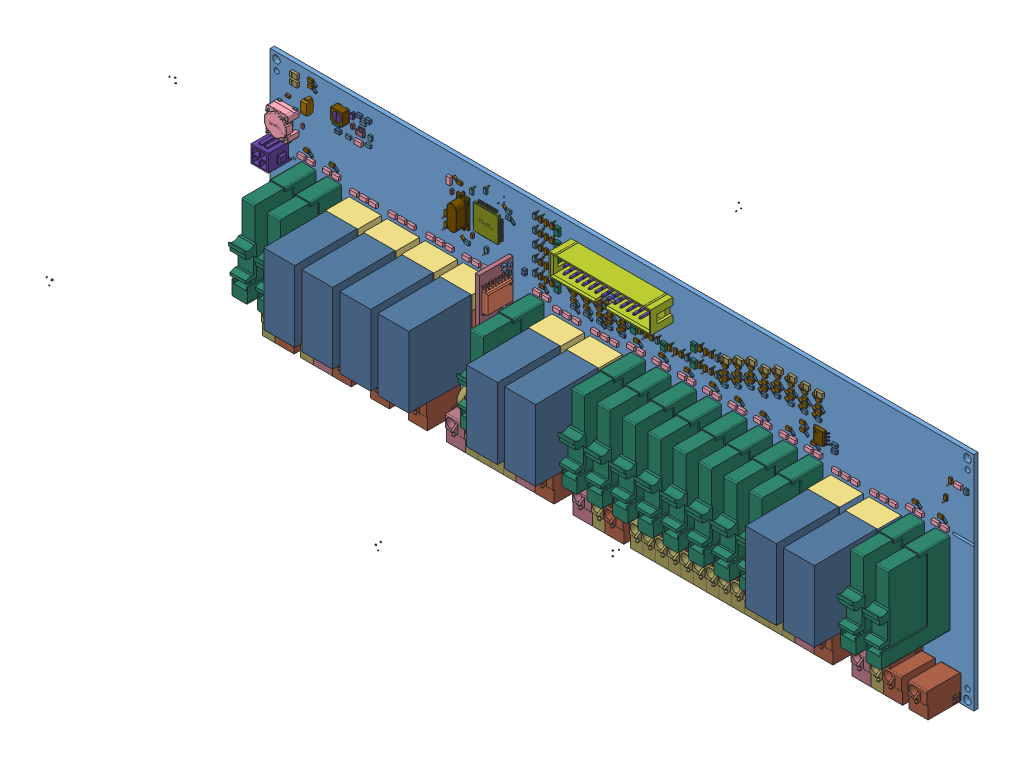
SolidWorks assembly _SC941C, configuration Default. Lengths in mm. (continued)
Components (placement in the parent): (continued)
- D33-1: D33 [Default] at origin size (1.9 2.9 0.99)
  - 1151710376-1: 1151710376 [Default] at (164.592 62.23 0) size (1.9 2.9 0.98)
    - Extruded-1: Extruded [Default] at origin size (1.9 2.9 0.98)
  - 1151710512-1: 1151710512 [Default] at (164.592 62.865 0.95) size (1.78 0.25 0.04)
    - Extruded_1-1: Extruded_1 [Default] at origin size (1.78 0.25 0.04)
- D31-1: D31 [Default] at origin size (1.9 2.9 0.99)
  - 1151710376-1: 1151710376 [Default] at (164.465 56.388 0) size (1.9 2.9 0.98)
    - Extruded-1: Extruded [Default] at origin size (1.9 2.9 0.98)
  - 1151710512-1: 1151710512 [Default] at (164.465 57.023 0.95) size (1.78 0.25 0.04)
    - Extruded_1-1: Extruded_1 [Default] at origin size (1.78 0.25 0.04)
- D29-1: D29 [Default] at origin size (1.9 2.9 0.99)
  - 1151710376-1: 1151710376 [Default] at (152.527 56.388 0) size (1.9 2.9 0.98)
    - Extruded-1: Extruded [Default] at origin size (1.9 2.9 0.98)
  - 1151710512-1: 1151710512 [Default] at (152.527 57.023 0.95) size (1.78 0.25 0.04)
    - Extruded_1-1: Extruded_1 [Default] at origin size (1.78 0.25 0.04)
- D23-1: D23 [Default] at origin size (1.9 2.9 0.99)
  - 1151710376-1: 1151710376 [Default] at (140.589 56.388 0) size (1.9 2.9 0.98)
    - Extruded-1: Extruded [Default] at origin size (1.9 2.9 0.98)
  - 1151710512-1: 1151710512 [Default] at (140.589 57.023 0.95) size (1.78 0.25 0.04)
    - Extruded_1-1: Extruded_1 [Default] at origin size (1.78 0.25 0.04)
- D22-1: D22 [Default] at origin size (2.9 1.9 0.99)
  - 905269392-1: 905269392 [Default] at (131.318 61.087 0) size (2.9 1.9 0.98)
    - Extruded_17-1: Extruded_17 [Default] at origin size (2.9 1.9 0.98)
  - 905269800-1: 905269800 [Default] at (130.683 61.087 0.95) size (0.25 1.78 0.04)
    - Extruded_18-1: Extruded_18 [Default] at origin size (0.25 1.78 0.04)
- D20-1: D20 [Default] at origin size (2.9 1.9 0.99)
  - 905269392-1: 905269392 [Default] at (136.525 61.087 0) size (2.9 1.9 0.98)
    - Extruded_17-1: Extruded_17 [Default] at origin size (2.9 1.9 0.98)
  - 905269800-1: 905269800 [Default] at (135.89 61.087 0.95) size (0.25 1.78 0.04)
    - Extruded_18-1: Extruded_18 [Default] at origin size (0.25 1.78 0.04)
- D18-1: D18 [Default] at origin size (2.9 1.9 0.99)
  - 905269392-1: 905269392 [Default] at (126.111 61.087 0) size (2.9 1.9 0.98)
    - Extruded_17-1: Extruded_17 [Default] at origin size (2.9 1.9 0.98)
  - 905269800-1: 905269800 [Default] at (126.746 61.087 0.95) size (0.25 1.78 0.04)
    - Extruded_18-1: Extruded_18 [Default] at origin size (0.25 1.78 0.04)
- D12-1: D12 [Default] at origin size (2.9 1.9 0.99)
  - 905269392-1: 905269392 [Default] at (120.904 61.087 0) size (2.9 1.9 0.98)
    - Extruded_17-1: Extruded_17 [Default] at origin size (2.9 1.9 0.98)
  - 905269800-1: 905269800 [Default] at (121.539 61.087 0.95) size (0.25 1.78 0.04)
    - Extruded_18-1: Extruded_18 [Default] at origin size (0.25 1.78 0.04)
- D10-1: D10 [Default] at origin size (1.9 2.9 0.99)
  - 1151710376-1: 1151710376 [Default] at (109.855 60.198 0) size (1.9 2.9 0.98)
    - Extruded-1: Extruded [Default] at origin size (1.9 2.9 0.98)
  - 1151710512-1: 1151710512 [Default] at (109.855 60.833 0.95) size (1.78 0.25 0.04)
    - Extruded_1-1: Extruded_1 [Default] at origin size (1.78 0.25 0.04)
- D19-1: D19 [Default] at origin size (1.9 2.9 0.99)
  - 1151710376-1: 1151710376 [Default] at (109.855 55.245 0) size (1.9 2.9 0.98)
    - Extruded-1: Extruded [Default] at origin size (1.9 2.9 0.98)
  - 1151710512-1: 1151710512 [Default] at (109.855 55.88 0.95) size (1.78 0.25 0.04)
    - Extruded_1-1: Extruded_1 [Default] at origin size (1.78 0.25 0.04)
- D16-1: D16 [Default] at origin size (1.9 2.9 0.99)
  - 1151710376-1: 1151710376 [Default] at (109.855 75.057 0) size (1.9 2.9 0.98)
    - Extruded-1: Extruded [Default] at origin size (1.9 2.9 0.98)
  - 1151710512-1: 1151710512 [Default] at (109.855 75.692 0.95) size (1.78 0.25 0.04)
    - Extruded_1-1: Extruded_1 [Default] at origin size (1.78 0.25 0.04)
- D13-1: D13 [Default] at origin size (1.9 2.9 0.99)
  - 1151710376-1: 1151710376 [Default] at (109.855 65.151 0) size (1.9 2.9 0.98)
    - Extruded-1: Extruded [Default] at origin size (1.9 2.9 0.98)
  - 1151710512-1: 1151710512 [Default] at (109.855 65.786 0.95) size (1.78 0.25 0.04)
    - Extruded_1-1: Extruded_1 [Default] at origin size (1.78 0.25 0.04)
- D11-1: D11 [Default] at origin size (1.9 2.9 0.99)
  - 1151710376-1: 1151710376 [Default] at (109.855 70.104 0) size (1.9 2.9 0.98)
    - Extruded-1: Extruded [Default] at origin size (1.9 2.9 0.98)
  - 1151710512-1: 1151710512 [Default] at (109.855 70.739 0.95) size (1.78 0.25 0.04)
    - Extruded_1-1: Extruded_1 [Default] at origin size (1.78 0.25 0.04)
- D32-1: D32 [Default] at origin size (104.77 29.62 23.48)
  - SW3dPS-transistor_SOT233_4-1: SW3dPS-transistor_SOT233_4 [Default] at (101.3713 26.7469 -21.9) x (-1 0 0) z (0 1 0) size (2.9 1.1 1.6)
  - SW3dPS-transistor_SOT233_5-1: SW3dPS-transistor_SOT233_5 [Default] at (0.1014 0.0267 -0.0219) x (-1 0 0) z (0 1 0) size (2.18 2.18 2.18)
  - SW3dPS-transistor_SOT233_6-1: SW3dPS-transistor_SOT233_6 [Default] at (0.0001 0 0) x (-1 0 0) z (0 1 0) size (2.18 2.18 2.18)
  - SW3dPS-transistor_SOT233_7-1: SW3dPS-transistor_SOT233_7 [Default] x (-1 0 0) z (0 1 0) size (2.18 2.18 2.18)
- D30-1: D30 [Default] at origin size (94.62 29.62 23.48)
  - SW3dPS-transistor_SOT233_4-1: SW3dPS-transistor_SOT233_4 [Default] at (91.2113 26.7469 -21.9) x (-1 0 0) z (0 1 0) size (2.9 1.1 1.6)
  - SW3dPS-transistor_SOT233_5-1: SW3dPS-transistor_SOT233_5 [Default] at (0.0912 0.0267 -0.0219) x (-1 0 0) z (0 1 0) size (2.18 2.18 2.18)
  - SW3dPS-transistor_SOT233_6-1: SW3dPS-transistor_SOT233_6 [Default] at (0.0001 0 0) x (-1 0 0) z (0 1 0) size (2.18 2.18 2.18)
  - SW3dPS-transistor_SOT233_7-1: SW3dPS-transistor_SOT233_7 [Default] x (-1 0 0) z (0 1 0) size (2.18 2.18 2.18)
- D48-1: D48 [Default] at origin size (2.9 1.9 0.99)
  - 905269392-1: 905269392 [Default] at (193.294 68.707 0) size (2.9 1.9 0.98)
    - Extruded_17-1: Extruded_17 [Default] at origin size (2.9 1.9 0.98)
  - 905269800-1: 905269800 [Default] at (192.659 68.707 0.95) size (0.25 1.78 0.04)
    - Extruded_18-1: Extruded_18 [Default] at origin size (0.25 1.78 0.04)
- D46-1: D46 [Default] at origin size (2.9 1.9 0.99)
  - 905269392-1: 905269392 [Default] at (198.501 70.993 0) size (2.9 1.9 0.98)
    - Extruded_17-1: Extruded_17 [Default] at origin size (2.9 1.9 0.98)
  - 905269800-1: 905269800 [Default] at (197.866 70.993 0.95) size (0.25 1.78 0.04)
    - Extruded_18-1: Extruded_18 [Default] at origin size (0.25 1.78 0.04)
- D44-1: D44 [Default] at origin size (171.7 27.55 23.48)
  - SW3dPS-transistor_SOT233_4-1: SW3dPS-transistor_SOT233_4 [Default] at (168.3638 24.6832 -21.9) x (-1 0 0) z (0 1 0) size (2.9 1.1 1.6)
  - SW3dPS-transistor_SOT233_5-1: SW3dPS-transistor_SOT233_5 [Default] at (0.1684 0.0247 -0.0219) x (-1 0 0) z (0 1 0) size (2.18 2.18 2.18)
  - SW3dPS-transistor_SOT233_6-1: SW3dPS-transistor_SOT233_6 [Default] at (0.0002 0 0) x (-1 0 0) z (0 1 0) size (2.18 2.18 2.18)
  - SW3dPS-transistor_SOT233_7-1: SW3dPS-transistor_SOT233_7 [Default] x (-1 0 0) z (0 1 0) size (2.18 2.18 2.18)
- D42-1: D42 [Default] at origin size (156.47 27.55 23.48)
  - SW3dPS-transistor_SOT233_4-1: SW3dPS-transistor_SOT233_4 [Default] at (153.1238 24.6832 -21.9) x (-1 0 0) z (0 1 0) size (2.9 1.1 1.6)
  - SW3dPS-transistor_SOT233_5-1: SW3dPS-transistor_SOT233_5 [Default] at (0.1531 0.0247 -0.0219) x (-1 0 0) z (0 1 0) size (2.18 2.18 2.18)
  - SW3dPS-transistor_SOT233_6-1: SW3dPS-transistor_SOT233_6 [Default] at (0.0002 0 0) x (-1 0 0) z (0 1 0) size (2.18 2.18 2.18)
  - SW3dPS-transistor_SOT233_7-1: SW3dPS-transistor_SOT233_7 [Default] x (-1 0 0) z (0 1 0) size (2.18 2.18 2.18)
- D26-1: D26 [Default] at origin size (60.05 27.6 23.48)
  - SW3dPS-transistor_SOT233_4-1: SW3dPS-transistor_SOT233_4 [Default] at (56.6038 24.7282 -21.9) x (-1 0 0) z (0 1 0) size (2.9 1.1 1.6)
  - SW3dPS-transistor_SOT233_5-1: SW3dPS-transistor_SOT233_5 [Default] at (0.0566 0.0247 -0.0219) x (-1 0 0) z (0 1 0) size (2.18 2.18 2.18)
  - SW3dPS-transistor_SOT233_6-1: SW3dPS-transistor_SOT233_6 [Default] at (0.0001 0 0) x (-1 0 0) z (0 1 0) size (2.18 2.18 2.18)
  - SW3dPS-transistor_SOT233_7-1: SW3dPS-transistor_SOT233_7 [Default] x (-1 0 0) z (0 1 0) size (2.18 2.18 2.18)
- D25-1: D25 [Default] at origin size (44.82 27.6 23.48)
  - SW3dPS-transistor_SOT233_4-1: SW3dPS-transistor_SOT233_4 [Default] at (41.3638 24.7282 -21.9) x (-1 0 0) z (0 1 0) size (2.9 1.1 1.6)
  - SW3dPS-transistor_SOT233_5-1: SW3dPS-transistor_SOT233_5 [Default] at (0.0414 0.0247 -0.0219) x (-1 0 0) z (0 1 0) size (2.18 2.18 2.18)
  - SW3dPS-transistor_SOT233_6-1: SW3dPS-transistor_SOT233_6 [Default] at (0 0 0) x (-1 0 0) z (0 1 0) size (2.18 2.18 2.18)
  - SW3dPS-transistor_SOT233_7-1: SW3dPS-transistor_SOT233_7 [Default] x (-1 0 0) z (0 1 0) size (2.18 2.18 2.18)
- D21-1: D21 [Default] at origin size (8.51 27.6 23.48)
  - SW3dPS-transistor_SOT233_4-1: SW3dPS-transistor_SOT233_4 [Default] at (5.0101 24.7282 -21.9) x (-1 0 0) z (0 1 0) size (2.9 1.1 1.6)
  - SW3dPS-transistor_SOT233_5-1: SW3dPS-transistor_SOT233_5 [Default] at (0.005 0.0247 -0.0219) x (-1 0 0) z (0 1 0) size (2.18 2.18 2.18)
  - SW3dPS-transistor_SOT233_6-1: SW3dPS-transistor_SOT233_6 [Default] at (0 0 0) x (-1 0 0) z (0 1 0) size (2.18 2.18 2.18)
  - SW3dPS-transistor_SOT233_7-1: SW3dPS-transistor_SOT233_7 [Default] x (-1 0 0) z (0 1 0) size (2.18 2.18 2.18)
- D17-1: D17 [Default] at origin size (12.91 27.55 23.48)
  - SW3dPS-transistor_SOT233_4-1: SW3dPS-transistor_SOT233_4 [Default] at (-9.4362 24.6832 -21.9) x (-1 0 0) z (0 1 0) size (2.9 1.1 1.6)
  - SW3dPS-transistor_SOT233_5-1: SW3dPS-transistor_SOT233_5 [Default] at (-0.0094 0.0247 -0.0219) x (-1 0 0) z (0 1 0) size (2.18 2.18 2.18)
  - SW3dPS-transistor_SOT233_6-1: SW3dPS-transistor_SOT233_6 [Default] at (0 0 0) x (-1 0 0) z (0 1 0) size (2.18 2.18 2.18)
  - SW3dPS-transistor_SOT233_7-1: SW3dPS-transistor_SOT233_7 [Default] x (-1 0 0) z (0 1 0) size (2.18 2.18 2.18)
- D14-1: D14 [Default] at origin size (28.15 27.55 23.48)
  - SW3dPS-transistor_SOT233_4-1: SW3dPS-transistor_SOT233_4 [Default] at (-24.6762 24.6832 -21.9) x (-1 0 0) z (0 1 0) size (2.9 1.1 1.6)
  - SW3dPS-transistor_SOT233_5-1: SW3dPS-transistor_SOT233_5 [Default] at (-0.0247 0.0247 -0.0219) x (-1 0 0) z (0 1 0) size (2.18 2.18 2.18)
  - SW3dPS-transistor_SOT233_6-1: SW3dPS-transistor_SOT233_6 [Default] at (0 0 0) x (-1 0 0) z (0 1 0) size (2.18 2.18 2.18)
  - SW3dPS-transistor_SOT233_7-1: SW3dPS-transistor_SOT233_7 [Default] x (-1 0 0) z (0 1 0) size (2.18 2.18 2.18)
- D9-1: D9 [Default] at origin size (43.39 27.55 23.48)
  - SW3dPS-transistor_SOT233_4-1: SW3dPS-transistor_SOT233_4 [Default] at (-39.9162 24.6832 -21.9) x (-1 0 0) z (0 1 0) size (2.9 1.1 1.6)
  - SW3dPS-transistor_SOT233_5-1: SW3dPS-transistor_SOT233_5 [Default] at (-0.0399 0.0247 -0.0219) x (-1 0 0) z (0 1 0) size (2.18 2.18 2.18)
  - SW3dPS-transistor_SOT233_6-1: SW3dPS-transistor_SOT233_6 [Default] at (0 0 0) x (-1 0 0) z (0 1 0) size (2.18 2.18 2.18)
  - SW3dPS-transistor_SOT233_7-1: SW3dPS-transistor_SOT233_7 [Default] x (-1 0 0) z (0 1 0) size (2.18 2.18 2.18)
- C26-1: C26 [Default] at origin size (1.97 3.3 0.78)
  - SW3dPS-0805_SMD_Capacitor-1: SW3dPS-0805_SMD_Capacitor [Default] at (67.437 58.9279 0) x (0 -1 0) z (-1 0 0) size (2 0.78 1.25)
  - 905260688-1: 905260688 [Default] at (68.072 60.5949 0) size (1.43 1.11 0.76)
    - Extruded_13-1: Extruded_13 [Default] at origin size (1.43 1.11 0.76)
  - 905261368-1: 905261368 [Default] at (68.0323 60.4758 0) size (1.51 1.51 0.76)
    - Extruded_12-1: Extruded_12 [Default] at origin size (1.51 1.51 0.76)
  - 905262864-1: 905262864 [Default] at (68.1117 60.7139 0) size (1.35 1.03 0.76)
    - Extruded_11-1: Extruded_11 [Default] at origin size (1.35 1.03 0.76)
- C24-1: C24 [Default] at origin size (1.97 3.3 0.78)
  - SW3dPS-0805_SMD_Capacitor-1: SW3dPS-0805_SMD_Capacitor [Default] at (67.437 54.8639 0) x (0 -1 0) z (-1 0 0) size (2 0.78 1.25)
  - 905260688-1: 905260688 [Default] at (68.072 56.5309 0) size (1.43 1.11 0.76)
    - Extruded_13-1: Extruded_13 [Default] at origin size (1.43 1.11 0.76)
  - 905261368-1: 905261368 [Default] at (68.0323 56.4118 0) size (1.51 1.51 0.76)
    - Extruded_12-1: Extruded_12 [Default] at origin size (1.51 1.51 0.76)
  - 905262864-1: 905262864 [Default] at (68.1117 56.6499 0) size (1.35 1.03 0.76)
    - Extruded_11-1: Extruded_11 [Default] at origin size (1.35 1.03 0.76)
- C17-1: C17 [Default] at origin size (3.3 1.97 0.78)
  - SW3dPS-0805_SMD_Capacitor-1: SW3dPS-0805_SMD_Capacitor [Default] at (90.2971 72.009 0) x (1 0 0) z (0 -1 0) size (2 0.78 1.25)
  - 905266536-1: 905266536 [Default] at (88.6301 72.644 0) size (1.11 1.43 0.76)
    - Extruded_16-1: Extruded_16 [Default] at origin size (1.11 1.43 0.76)
  - 905263816-1: 905263816 [Default] at (88.7492 72.6043 0) size (1.51 1.51 0.76)
    - Extruded_15-1: Extruded_15 [Default] at origin size (1.51 1.51 0.76)
  - 905266264-1: 905266264 [Default] at (88.5111 72.6837 0) size (1.03 1.35 0.76)
    - Extruded_14-1: Extruded_14 [Default] at origin size (1.03 1.35 0.76)
- C19-1: C19 [Default] at origin size (1.97 3.3 0.78)
  - SW3dPS-0805_SMD_Capacitor-1: SW3dPS-0805_SMD_Capacitor [Default] at (81.0298 74.5344 0) x (0 -1 0) z (-1 0 0) size (2 0.78 1.25)
  - 905260688-1: 905260688 [Default] at (81.6648 76.2014 0) size (1.43 1.11 0.76)
    - Extruded_13-1: Extruded_13 [Default] at origin size (1.43 1.11 0.76)
  - 905261368-1: 905261368 [Default] at (81.6251 76.0823 0) size (1.51 1.51 0.76)
    - Extruded_12-1: Extruded_12 [Default] at origin size (1.51 1.51 0.76)
  - 905262864-1: 905262864 [Default] at (81.7045 76.3204 0) size (1.35 1.03 0.76)
    - Extruded_11-1: Extruded_11 [Default] at origin size (1.35 1.03 0.76)
- C25-1: C25 [Default] at origin size (3.3 1.97 0.78)
  - SW3dPS-0805_SMD_Capacitor-1: SW3dPS-0805_SMD_Capacitor [Default] at (90.2969 69.723 0) x (-1 0 0) z (0 1 0) size (2 0.78 1.25)
  - 905265720-1: 905265720 [Default] at (91.9639 69.088 0) size (1.11 1.43 0.76)
    - Extruded_4-1: Extruded_4 [Default] at origin size (1.11 1.43 0.76)
  - 905275240-1: 905275240 [Default] at (91.8448 69.1277 0) size (1.51 1.51 0.76)
    - Extruded_3-1: Extruded_3 [Default] at origin size (1.51 1.51 0.76)
  - 905261096-1: 905261096 [Default] at (92.0829 69.0483 0) size (1.03 1.35 0.76)
    - Extruded_2-1: Extruded_2 [Default] at origin size (1.03 1.35 0.76)
- C21-1: C21 [Default] at origin size (3.3 1.97 0.78)
  - SW3dPS-0805_SMD_Capacitor-1: SW3dPS-0805_SMD_Capacitor [Default] at (73.6601 52.832 0) x (1 0 0) z (0 -1 0) size (2 0.78 1.25)
  - 905266536-1: 905266536 [Default] at (71.9931 53.467 0) size (1.11 1.43 0.76)
    - Extruded_16-1: Extruded_16 [Default] at origin size (1.11 1.43 0.76)
  - 905263816-1: 905263816 [Default] at (72.1122 53.4273 0) size (1.51 1.51 0.76)
    - Extruded_15-1: Extruded_15 [Default] at origin size (1.51 1.51 0.76)
  - 905266264-1: 905266264 [Default] at (71.8741 53.5067 0) size (1.03 1.35 0.76)
    - Extruded_14-1: Extruded_14 [Default] at origin size (1.03 1.35 0.76)
- C18-1: C18 [Default] at origin size (1.97 3.3 0.78)
  - SW3dPS-0805_SMD_Capacitor-1: SW3dPS-0805_SMD_Capacitor [Default] at (75.4736 71.5181 0) x (0 -1 0) z (-1 0 0) size (2 0.78 1.25)
  - 905260688-1: 905260688 [Default] at (76.1086 73.1851 0) size (1.43 1.11 0.76)
    - Extruded_13-1: Extruded_13 [Default] at origin size (1.43 1.11 0.76)
  - 905261368-1: 905261368 [Default] at (76.0689 73.066 0) size (1.51 1.51 0.76)
    - Extruded_12-1: Extruded_12 [Default] at origin size (1.51 1.51 0.76)
  - 905262864-1: 905262864 [Default] at (76.1483 73.3041 0) size (1.35 1.03 0.76)
    - Extruded_11-1: Extruded_11 [Default] at origin size (1.35 1.03 0.76)
- C20-1: C20 [Default] at origin size (1.97 3.3 0.78)
  - SW3dPS-0805_SMD_Capacitor-1: SW3dPS-0805_SMD_Capacitor [Default] at (81.3473 54.1828 0) x (0 1 0) z (1 0 0) size (2 0.78 1.25)
  - 905266128-1: 905266128 [Default] at (80.7123 52.5158 0) size (1.43 1.11 0.76)
    - Extruded_10-1: Extruded_10 [Default] at origin size (1.43 1.11 0.76)
  - 905260416-1: 905260416 [Default] at (80.752 52.6349 0) size (1.51 1.51 0.76)
    - Extruded_9-1: Extruded_9 [Default] at origin size (1.51 1.51 0.76)
  - 905261640-1: 905261640 [Default] at (80.6726 52.3968 0) size (1.35 1.03 0.76)
    - Extruded_8-1: Extruded_8 [Default] at origin size (1.35 1.03 0.76)
- C37-1: C37 [Default] at origin size (3.3 1.97 0.78)
  - SW3dPS-0805_SMD_Capacitor-1: SW3dPS-0805_SMD_Capacitor [Default] at (192.7861 59.563 0) x (1 0 0) z (0 -1 0) size (2 0.78 1.25)
  - 905266536-1: 905266536 [Default] at (191.1191 60.198 0) size (1.11 1.43 0.76)
    - Extruded_16-1: Extruded_16 [Default] at origin size (1.11 1.43 0.76)
  - 905263816-1: 905263816 [Default] at (191.2382 60.1583 0) size (1.51 1.51 0.76)
    - Extruded_15-1: Extruded_15 [Default] at origin size (1.51 1.51 0.76)
  - 905266264-1: 905266264 [Default] at (191.0001 60.2377 0) size (1.03 1.35 0.76)
    - Extruded_14-1: Extruded_14 [Default] at origin size (1.03 1.35 0.76)
- C36-1: C36 [Default] at origin size (3.3 1.97 0.78)
  - SW3dPS-0805_SMD_Capacitor-1: SW3dPS-0805_SMD_Capacitor [Default] at (197.9931 61.849 0) x (1 0 0) z (0 -1 0) size (2 0.78 1.25)
  - 905266536-1: 905266536 [Default] at (196.3261 62.484 0) size (1.11 1.43 0.76)
    - Extruded_16-1: Extruded_16 [Default] at origin size (1.11 1.43 0.76)
  - 905263816-1: 905263816 [Default] at (196.4452 62.4443 0) size (1.51 1.51 0.76)
    - Extruded_15-1: Extruded_15 [Default] at origin size (1.51 1.51 0.76)
  - 905266264-1: 905266264 [Default] at (196.2071 62.5237 0) size (1.03 1.35 0.76)
    - Extruded_14-1: Extruded_14 [Default] at origin size (1.03 1.35 0.76)
- C35-1: C35 [Default] at origin size (3.3 1.97 0.78)
  - SW3dPS-0805_SMD_Capacitor-1: SW3dPS-0805_SMD_Capacitor [Default] at (187.3251 59.563 0) x (1 0 0) z (0 -1 0) size (2 0.78 1.25)
  - 905266536-1: 905266536 [Default] at (185.6581 60.198 0) size (1.11 1.43 0.76)
    - Extruded_16-1: Extruded_16 [Default] at origin size (1.11 1.43 0.76)
  - 905263816-1: 905263816 [Default] at (185.7772 60.1583 0) size (1.51 1.51 0.76)
    - Extruded_15-1: Extruded_15 [Default] at origin size (1.51 1.51 0.76)
  - 905266264-1: 905266264 [Default] at (185.5391 60.2377 0) size (1.03 1.35 0.76)
    - Extruded_14-1: Extruded_14 [Default] at origin size (1.03 1.35 0.76)
- C34-1: C34 [Default] at origin size (3.3 1.97 0.78)
  - SW3dPS-0805_SMD_Capacitor-1: SW3dPS-0805_SMD_Capacitor [Default] at (203.4541 61.849 0) x (1 0 0) z (0 -1 0) size (2 0.78 1.25)
  - 905266536-1: 905266536 [Default] at (201.7871 62.484 0) size (1.11 1.43 0.76)
    - Extruded_16-1: Extruded_16 [Default] at origin size (1.11 1.43 0.76)
  - 905263816-1: 905263816 [Default] at (201.9062 62.4443 0) size (1.51 1.51 0.76)
    - Extruded_15-1: Extruded_15 [Default] at origin size (1.51 1.51 0.76)
  - 905266264-1: 905266264 [Default] at (201.6681 62.5237 0) size (1.03 1.35 0.76)
    - Extruded_14-1: Extruded_14 [Default] at origin size (1.03 1.35 0.76)
- C33-1: C33 [Default] at origin size (3.3 1.97 0.78)
  - SW3dPS-0805_SMD_Capacitor-1: SW3dPS-0805_SMD_Capacitor [Default] at (182.1181 57.277 0) x (1 0 0) z (0 -1 0) size (2 0.78 1.25)
  - 905266536-1: 905266536 [Default] at (180.4511 57.912 0) size (1.11 1.43 0.76)
    - Extruded_16-1: Extruded_16 [Default] at origin size (1.11 1.43 0.76)
  - 905263816-1: 905263816 [Default] at (180.5702 57.8723 0) size (1.51 1.51 0.76)
    - Extruded_15-1: Extruded_15 [Default] at origin size (1.51 1.51 0.76)
  - 905266264-1: 905266264 [Default] at (180.3321 57.9517 0) size (1.03 1.35 0.76)
    - Extruded_14-1: Extruded_14 [Default] at origin size (1.03 1.35 0.76)
- C32-1: C32 [Default] at origin size (3.3 1.97 0.78)
  - SW3dPS-0805_SMD_Capacitor-1: SW3dPS-0805_SMD_Capacitor [Default] at (208.9151 61.849 0) x (1 0 0) z (0 -1 0) size (2 0.78 1.25)
  - 905266536-1: 905266536 [Default] at (207.2481 62.484 0) size (1.11 1.43 0.76)
    - Extruded_16-1: Extruded_16 [Default] at origin size (1.11 1.43 0.76)
  - 905263816-1: 905263816 [Default] at (207.3672 62.4443 0) size (1.51 1.51 0.76)
    - Extruded_15-1: Extruded_15 [Default] at origin size (1.51 1.51 0.76)
  - 905266264-1: 905266264 [Default] at (207.1291 62.5237 0) size (1.03 1.35 0.76)
    - Extruded_14-1: Extruded_14 [Default] at origin size (1.03 1.35 0.76)
- C31-1: C31 [Default] at origin size (3.3 1.97 0.78)
  - SW3dPS-0805_SMD_Capacitor-1: SW3dPS-0805_SMD_Capacitor [Default] at (176.9111 54.991 0) x (1 0 0) z (0 -1 0) size (2 0.78 1.25)
  - 905266536-1: 905266536 [Default] at (175.2441 55.626 0) size (1.11 1.43 0.76)
    - Extruded_16-1: Extruded_16 [Default] at origin size (1.11 1.43 0.76)
  - 905263816-1: 905263816 [Default] at (175.3632 55.5863 0) size (1.51 1.51 0.76)
    - Extruded_15-1: Extruded_15 [Default] at origin size (1.51 1.51 0.76)
  - 905266264-1: 905266264 [Default] at (175.1251 55.6657 0) size (1.03 1.35 0.76)
    - Extruded_14-1: Extruded_14 [Default] at origin size (1.03 1.35 0.76)
- C30-1: C30 [Default] at origin size (3.3 1.97 0.78)
  - SW3dPS-0805_SMD_Capacitor-1: SW3dPS-0805_SMD_Capacitor [Default] at (214.3761 61.849 0) x (1 0 0) z (0 -1 0) size (2 0.78 1.25)
  - 905266536-1: 905266536 [Default] at (212.7091 62.484 0) size (1.11 1.43 0.76)
    - Extruded_16-1: Extruded_16 [Default] at origin size (1.11 1.43 0.76)
  - 905263816-1: 905263816 [Default] at (212.8282 62.4443 0) size (1.51 1.51 0.76)
    - Extruded_15-1: Extruded_15 [Default] at origin size (1.51 1.51 0.76)
  - 905266264-1: 905266264 [Default] at (212.5901 62.5237 0) size (1.03 1.35 0.76)
    - Extruded_14-1: Extruded_14 [Default] at origin size (1.03 1.35 0.76)
- C29-1: C29 [Default] at origin size (1.97 3.3 0.78)
  - SW3dPS-0805_SMD_Capacitor-1: SW3dPS-0805_SMD_Capacitor [Default] at (173.736 62.7379 0) x (0 -1 0) z (-1 0 0) size (2 0.78 1.25)
  - 905260688-1: 905260688 [Default] at (174.371 64.4049 0) size (1.43 1.11 0.76)
    - Extruded_13-1: Extruded_13 [Default] at origin size (1.43 1.11 0.76)
  - 905261368-1: 905261368 [Default] at (174.3313 64.2858 0) size (1.51 1.51 0.76)
    - Extruded_12-1: Extruded_12 [Default] at origin size (1.51 1.51 0.76)
  - 905262864-1: 905262864 [Default] at (174.4107 64.5239 0) size (1.35 1.03 0.76)
    - Extruded_11-1: Extruded_11 [Default] at origin size (1.35 1.03 0.76)
- C28-1: C28 [Default] at origin size (1.97 3.3 0.78)
  - SW3dPS-0805_SMD_Capacitor-1: SW3dPS-0805_SMD_Capacitor [Default] at (173.609 56.8959 0) x (0 -1 0) z (-1 0 0) size (2 0.78 1.25)
  - 905260688-1: 905260688 [Default] at (174.244 58.5629 0) size (1.43 1.11 0.76)
    - Extruded_13-1: Extruded_13 [Default] at origin size (1.43 1.11 0.76)
  - 905261368-1: 905261368 [Default] at (174.2043 58.4438 0) size (1.51 1.51 0.76)
    - Extruded_12-1: Extruded_12 [Default] at origin size (1.51 1.51 0.76)
  - 905262864-1: 905262864 [Default] at (174.2837 58.6819 0) size (1.35 1.03 0.76)
    - Extruded_11-1: Extruded_11 [Default] at origin size (1.35 1.03 0.76)
- C16-1: C16 [Default] at origin size (1.97 3.3 0.78)
  - SW3dPS-0805_SMD_Capacitor-1: SW3dPS-0805_SMD_Capacitor [Default] at (149.733 56.8959 0) x (0 -1 0) z (-1 0 0) size (2 0.78 1.25)
  - 905260688-1: 905260688 [Default] at (150.368 58.5629 0) size (1.43 1.11 0.76)
    - Extruded_13-1: Extruded_13 [Default] at origin size (1.43 1.11 0.76)
  - 905261368-1: 905261368 [Default] at (150.3283 58.4438 0) size (1.51 1.51 0.76)
    - Extruded_12-1: Extruded_12 [Default] at origin size (1.51 1.51 0.76)
  - 905262864-1: 905262864 [Default] at (150.4077 58.6819 0) size (1.35 1.03 0.76)
    - Extruded_11-1: Extruded_11 [Default] at origin size (1.35 1.03 0.76)
- C14-1: C14 [Default] at origin size (3.3 1.97 0.78)
  - SW3dPS-0805_SMD_Capacitor-1: SW3dPS-0805_SMD_Capacitor [Default] at (130.8101 51.9431 0) x (1 0 0) z (0 -1 0) size (2 0.78 1.25)
  - 905266536-1: 905266536 [Default] at (129.1431 52.578 0) size (1.11 1.43 0.76)
    - Extruded_16-1: Extruded_16 [Default] at origin size (1.11 1.43 0.76)
  - 905263816-1: 905263816 [Default] at (129.2622 52.5383 0) size (1.51 1.51 0.76)
    - Extruded_15-1: Extruded_15 [Default] at origin size (1.51 1.51 0.76)
  - 905266264-1: 905266264 [Default] at (129.0241 52.6177 0) size (1.03 1.35 0.76)
    - Extruded_14-1: Extruded_14 [Default] at origin size (1.03 1.35 0.76)
- C13-1: C13 [Default] at origin size (3.3 1.97 0.78)
  - SW3dPS-0805_SMD_Capacitor-1: SW3dPS-0805_SMD_Capacitor [Default] at (136.0171 51.9431 0) x (1 0 0) z (0 -1 0) size (2 0.78 1.25)
  - 905266536-1: 905266536 [Default] at (134.3501 52.578 0) size (1.11 1.43 0.76)
    - Extruded_16-1: Extruded_16 [Default] at origin size (1.11 1.43 0.76)
  - 905263816-1: 905263816 [Default] at (134.4692 52.5383 0) size (1.51 1.51 0.76)
    - Extruded_15-1: Extruded_15 [Default] at origin size (1.51 1.51 0.76)
  - 905266264-1: 905266264 [Default] at (134.2311 52.6177 0) size (1.03 1.35 0.76)
    - Extruded_14-1: Extruded_14 [Default] at origin size (1.03 1.35 0.76)
- C7_1-1: C7_1 [Default] at origin size (3.3 1.97 0.78)
  - SW3dPS-0805_SMD_Capacitor-1: SW3dPS-0805_SMD_Capacitor [Default] at (121.4119 51.943 0) x (-1 0 0) z (0 1 0) size (2 0.78 1.25)
  - 905265720-1: 905265720 [Default] at (123.0789 51.308 0) size (1.11 1.43 0.76)
    - Extruded_4-1: Extruded_4 [Default] at origin size (1.11 1.43 0.76)
  - 905275240-1: 905275240 [Default] at (122.9598 51.3477 0) size (1.51 1.51 0.76)
    - Extruded_3-1: Extruded_3 [Default] at origin size (1.51 1.51 0.76)
  - 905261096-1: 905261096 [Default] at (123.1979 51.2683 0) size (1.03 1.35 0.76)
    - Extruded_2-1: Extruded_2 [Default] at origin size (1.03 1.35 0.76)
- C5_1-1: C5_1 [Default] at origin size (1.97 3.3 0.78)
  - SW3dPS-0805_SMD_Capacitor-1: SW3dPS-0805_SMD_Capacitor [Default] at (100.711 60.7059 0) x (0 -1 0) z (-1 0 0) size (2 0.78 1.25)
  - 905260688-1: 905260688 [Default] at (101.346 62.3729 0) size (1.43 1.11 0.76)
    - Extruded_13-1: Extruded_13 [Default] at origin size (1.43 1.11 0.76)
  - 905261368-1: 905261368 [Default] at (101.3063 62.2538 0) size (1.51 1.51 0.76)
    - Extruded_12-1: Extruded_12 [Default] at origin size (1.51 1.51 0.76)
  - 905262864-1: 905262864 [Default] at (101.3857 62.4919 0) size (1.35 1.03 0.76)
    - Extruded_11-1: Extruded_11 [Default] at origin size (1.35 1.03 0.76)
- C27-1: C27 [Default] at origin size (1.97 3.3 0.78)
  - SW3dPS-0805_SMD_Capacitor-1: SW3dPS-0805_SMD_Capacitor [Default] at (161.671 56.8959 0) x (0 -1 0) z (-1 0 0) size (2 0.78 1.25)
  - 905260688-1: 905260688 [Default] at (162.306 58.5629 0) size (1.43 1.11 0.76)
    - Extruded_13-1: Extruded_13 [Default] at origin size (1.43 1.11 0.76)
  - 905261368-1: 905261368 [Default] at (162.2663 58.4438 0) size (1.51 1.51 0.76)
    - Extruded_12-1: Extruded_12 [Default] at origin size (1.51 1.51 0.76)
  - 905262864-1: 905262864 [Default] at (162.3457 58.6819 0) size (1.35 1.03 0.76)
    - Extruded_11-1: Extruded_11 [Default] at origin size (1.35 1.03 0.76)
- C11-1: C11 [Default] at origin size (3.3 1.97 0.78)
  - SW3dPS-0805_SMD_Capacitor-1: SW3dPS-0805_SMD_Capacitor [Default] at (126.6189 51.943 0) x (-1 0 0) z (0 1 0) size (2 0.78 1.25)
  - 905265720-1: 905265720 [Default] at (128.2859 51.308 0) size (1.11 1.43 0.76)
    - Extruded_4-1: Extruded_4 [Default] at origin size (1.11 1.43 0.76)
  - 905275240-1: 905275240 [Default] at (128.1668 51.3477 0) size (1.51 1.51 0.76)
    - Extruded_3-1: Extruded_3 [Default] at origin size (1.51 1.51 0.76)
  - 905261096-1: 905261096 [Default] at (128.4049 51.2683 0) size (1.03 1.35 0.76)
    - Extruded_2-1: Extruded_2 [Default] at origin size (1.03 1.35 0.76)
- C12-1: C12 [Default] at origin size (1.97 3.3 0.78)
  - SW3dPS-0805_SMD_Capacitor-1: SW3dPS-0805_SMD_Capacitor [Default] at (100.711 55.7529 0) x (0 -1 0) z (-1 0 0) size (2 0.78 1.25)
  - 905260688-1: 905260688 [Default] at (101.346 57.4199 0) size (1.43 1.11 0.76)
    - Extruded_13-1: Extruded_13 [Default] at origin size (1.43 1.11 0.76)
  - 905261368-1: 905261368 [Default] at (101.3063 57.3008 0) size (1.51 1.51 0.76)
    - Extruded_12-1: Extruded_12 [Default] at origin size (1.51 1.51 0.76)
  - 905262864-1: 905262864 [Default] at (101.3857 57.5389 0) size (1.35 1.03 0.76)
    - Extruded_11-1: Extruded_11 [Default] at origin size (1.35 1.03 0.76)
- C10-1: C10 [Default] at origin size (1.97 3.3 0.78)
  - SW3dPS-0805_SMD_Capacitor-1: SW3dPS-0805_SMD_Capacitor [Default] at (100.711 75.5649 0) x (0 -1 0) z (-1 0 0) size (2 0.78 1.25)
  - 905260688-1: 905260688 [Default] at (101.346 77.2319 0) size (1.43 1.11 0.76)
    - Extruded_13-1: Extruded_13 [Default] at origin size (1.43 1.11 0.76)
  - 905261368-1: 905261368 [Default] at (101.3063 77.1128 0) size (1.51 1.51 0.76)
    - Extruded_12-1: Extruded_12 [Default] at origin size (1.51 1.51 0.76)
  - 905262864-1: 905262864 [Default] at (101.3857 77.3509 0) size (1.35 1.03 0.76)
    - Extruded_11-1: Extruded_11 [Default] at origin size (1.35 1.03 0.76)
- C8_1-1: C8_1 [Default] at origin size (1.97 3.3 0.78)
  - SW3dPS-0805_SMD_Capacitor-1: SW3dPS-0805_SMD_Capacitor [Default] at (100.711 65.6589 0) x (0 -1 0) z (-1 0 0) size (2 0.78 1.25)
  - 905260688-1: 905260688 [Default] at (101.346 67.3259 0) size (1.43 1.11 0.76)
    - Extruded_13-1: Extruded_13 [Default] at origin size (1.43 1.11 0.76)
  - 905261368-1: 905261368 [Default] at (101.3063 67.2068 0) size (1.51 1.51 0.76)
    - Extruded_12-1: Extruded_12 [Default] at origin size (1.51 1.51 0.76)
  - 905262864-1: 905262864 [Default] at (101.3857 67.4449 0) size (1.35 1.03 0.76)
    - Extruded_11-1: Extruded_11 [Default] at origin size (1.35 1.03 0.76)
- C6_1-1: C6_1 [Default] at origin size (1.97 3.3 0.78)
  - SW3dPS-0805_SMD_Capacitor-1: SW3dPS-0805_SMD_Capacitor [Default] at (100.711 70.6119 0) x (0 -1 0) z (-1 0 0) size (2 0.78 1.25)
  - 905260688-1: 905260688 [Default] at (101.346 72.2789 0) size (1.43 1.11 0.76)
    - Extruded_13-1: Extruded_13 [Default] at origin size (1.43 1.11 0.76)
  - 905261368-1: 905261368 [Default] at (101.3063 72.1598 0) size (1.51 1.51 0.76)
    - Extruded_12-1: Extruded_12 [Default] at origin size (1.51 1.51 0.76)
  - 905262864-1: 905262864 [Default] at (101.3857 72.3979 0) size (1.35 1.03 0.76)
    - Extruded_11-1: Extruded_11 [Default] at origin size (1.35 1.03 0.76)
- D7_1-1: D7_1 [Default] at origin size (64.67 29.62 23.48)
  - SW3dPS-transistor_SOT233_4-1: SW3dPS-transistor_SOT233_4 [Default] at (-61.1887 26.7469 -21.9) x (-1 0 0) z (0 1 0) size (2.9 1.1 1.6)
  - SW3dPS-transistor_SOT233_5-1: SW3dPS-transistor_SOT233_5 [Default] at (-0.0612 0.0267 -0.0219) x (-1 0 0) z (0 1 0) size (2.18 2.18 2.18)
  - SW3dPS-transistor_SOT233_6-1: SW3dPS-transistor_SOT233_6 [Default] at (-0.0001 0 0) x (-1 0 0) z (0 1 0) size (2.18 2.18 2.18)
  - SW3dPS-transistor_SOT233_7-1: SW3dPS-transistor_SOT233_7 [Default] x (-1 0 0) z (0 1 0) size (2.18 2.18 2.18)
- D8-1: D8 [Default] at origin size (54.51 29.62 23.48)
  - SW3dPS-transistor_SOT233_4-1: SW3dPS-transistor_SOT233_4 [Default] at (-51.0287 26.7469 -21.9) x (-1 0 0) z (0 1 0) size (2.9 1.1 1.6)
  - SW3dPS-transistor_SOT233_5-1: SW3dPS-transistor_SOT233_5 [Default] at (-0.051 0.0267 -0.0219) x (-1 0 0) z (0 1 0) size (2.18 2.18 2.18)
  - SW3dPS-transistor_SOT233_6-1: SW3dPS-transistor_SOT233_6 [Default] at (-0.0001 0 0) x (-1 0 0) z (0 1 0) size (2.18 2.18 2.18)
  - SW3dPS-transistor_SOT233_7-1: SW3dPS-transistor_SOT233_7 [Default] x (-1 0 0) z (0 1 0) size (2.18 2.18 2.18)
- D40-1: D40 [Default] at origin size (145.37 29.62 23.48)
  - SW3dPS-transistor_SOT233_4-1: SW3dPS-transistor_SOT233_4 [Default] at (142.0113 26.7469 -21.9) x (-1 0 0) z (0 1 0) size (2.9 1.1 1.6)
  - SW3dPS-transistor_SOT233_5-1: SW3dPS-transistor_SOT233_5 [Default] at (0.142 0.0267 -0.0219) x (-1 0 0) z (0 1 0) size (2.18 2.18 2.18)
  - SW3dPS-transistor_SOT233_6-1: SW3dPS-transistor_SOT233_6 [Default] at (0.0001 0 0) x (-1 0 0) z (0 1 0) size (2.18 2.18 2.18)
  - SW3dPS-transistor_SOT233_7-1: SW3dPS-transistor_SOT233_7 [Default] x (-1 0 0) z (0 1 0) size (2.18 2.18 2.18)
- D47-1: D47 [Default] at origin size (185.97 29.62 23.48)
  - SW3dPS-transistor_SOT233_4-1: SW3dPS-transistor_SOT233_4 [Default] at (182.6513 26.7469 -21.9) x (-1 0 0) z (0 1 0) size (2.9 1.1 1.6)
  - SW3dPS-transistor_SOT233_5-1: SW3dPS-transistor_SOT233_5 [Default] at (0.1827 0.0267 -0.0219) x (-1 0 0) z (0 1 0) size (2.18 2.18 2.18)
  - SW3dPS-transistor_SOT233_6-1: SW3dPS-transistor_SOT233_6 [Default] at (0.0002 0 0) x (-1 0 0) z (0 1 0) size (2.18 2.18 2.18)
  - SW3dPS-transistor_SOT233_7-1: SW3dPS-transistor_SOT233_7 [Default] x (-1 0 0) z (0 1 0) size (2.18 2.18 2.18)
- K7-1: K7 [Default] at origin size (6.2 33 32.7)
  - User_Library-93_11-1: User_Library-93_11 [Default] at (97.865 47.3038 0) x (0 -1 0) z (0 0 1) size (33 6.2 32.7)
- K20-1: K20 [Default] at origin size (6.2 33 32.7)
  - User_Library-93_11-1: User_Library-93_11 [Default] at (250.265 47.3038 0) x (0 -1 0) z (0 0 1) size (33 6.2 32.7)
- K21-1: K21 [Default] at origin size (6.2 33 32.7)
  - User_Library-93_11-1: User_Library-93_11 [Default] at (260.425 47.3038 0) x (0 -1 0) z (0 0 1) size (33 6.2 32.7)
- R63-1: R63 [Default] at origin size (3.3 1.97 0.78)
  - SW3dPS-0805_SMD_Resistor-1: SW3dPS-0805_SMD_Resistor [Default] at (192.2462 52.7049 0) x (-1 0 0) z (0 1 0) size (2 0.78 1.25)
  - 905265720-1: 905265720 [Default] at (193.9131 52.07 0) size (1.11 1.43 0.76)
    - Extruded_4-1: Extruded_4 [Default] at origin size (1.11 1.43 0.76)
  - 905275240-1: 905275240 [Default] at (193.7941 52.1097 0) size (1.51 1.51 0.76)
    - Extruded_3-1: Extruded_3 [Default] at origin size (1.51 1.51 0.76)
  - 905261096-1: 905261096 [Default] at (194.0322 52.0303 0) size (1.03 1.35 0.76)
    - Extruded_2-1: Extruded_2 [Default] at origin size (1.03 1.35 0.76)
- R66-1: R66 [Default] at origin size (3.3 1.97 0.78)
  - SW3dPS-0805_SMD_Resistor-1: SW3dPS-0805_SMD_Resistor [Default] at (202.4062 52.7049 0) x (-1 0 0) z (0 1 0) size (2 0.78 1.25)
  - 905265720-1: 905265720 [Default] at (204.0731 52.07 0) size (1.11 1.43 0.76)
    - Extruded_4-1: Extruded_4 [Default] at origin size (1.11 1.43 0.76)
  - 905275240-1: 905275240 [Default] at (203.9541 52.1097 0) size (1.51 1.51 0.76)
    - Extruded_3-1: Extruded_3 [Default] at origin size (1.51 1.51 0.76)
  - 905261096-1: 905261096 [Default] at (204.1922 52.0303 0) size (1.03 1.35 0.76)
    - Extruded_2-1: Extruded_2 [Default] at origin size (1.03 1.35 0.76)
- R85-1: R85 [Default] at origin size (3.3 1.97 0.78)
  - SW3dPS-0805_SMD_Resistor-1: SW3dPS-0805_SMD_Resistor [Default] at (253.2062 52.7049 0) x (-1 0 0) z (0 1 0) size (2 0.78 1.25)
  - 905265720-1: 905265720 [Default] at (254.8731 52.07 0) size (1.11 1.43 0.76)
    - Extruded_4-1: Extruded_4 [Default] at origin size (1.11 1.43 0.76)
  - 905275240-1: 905275240 [Default] at (254.7541 52.1097 0) size (1.51 1.51 0.76)
    - Extruded_3-1: Extruded_3 [Default] at origin size (1.51 1.51 0.76)
  - 905261096-1: 905261096 [Default] at (254.9922 52.0303 0) size (1.03 1.35 0.76)
    - Extruded_2-1: Extruded_2 [Default] at origin size (1.03 1.35 0.76)
- SUP_K8-1: SUP_K8 [Default] at origin size (13 30.3 9.5)
  - 1151724928-1: 1151724928 [Default] at (113.665 41.975 0) size (13 5.5 9.5)
    - Extruded_7-1: Extruded_7 [Default] at origin size (13 5.5 9.5)
  - 1151725064-1: 1151725064 [Default] at (113.665 34.225 5) size (13 10 4.5)
    - Extruded_6-1: Extruded_6 [Default] at origin size (13 10 4.5)
  - 1151724792-1: 1151724792 [Default] at (113.665 21.825 0) size (13 14.8 9.5)
    - Extruded_5-1: Extruded_5 [Default] at origin size (13 14.8 9.5)
- SUP_K9-1: SUP_K9 [Default] at origin size (13 30.3 9.5)
  - 1151724928-1: 1151724928 [Default] at (128.905 41.975 0) size (13 5.5 9.5)
    - Extruded_7-1: Extruded_7 [Default] at origin size (13 5.5 9.5)
  - 1151725064-1: 1151725064 [Default] at (128.905 34.225 5) size (13 10 4.5)
    - Extruded_6-1: Extruded_6 [Default] at origin size (13 10 4.5)
  - 1151724792-1: 1151724792 [Default] at (128.905 21.825 0) size (13 14.8 9.5)
    - Extruded_5-1: Extruded_5 [Default] at origin size (13 14.8 9.5)
- J2-1: J2 [Default] at origin size (10 8.67 12.42)
  - c-3-794630-4-g-3d-1: c-3-794630-4-g-3d [Default] at (-0.6349 28.3801 9.3) x (1 0 0) z (0 0 1) size (10 8.67 12.42)
- J1-1: J1 [Default] at origin size (10 8.67 12.42)
  - c-3-794630-4-g-3d-1: c-3-794630-4-g-3d [Default] at (-0.6351 49.3799 9.3) x (-1 0 0) z (0 0 1) size (10 8.67 12.42)
- C23-1: C23 [Default] at origin size (0.8 1.6 0.9)
  - User_Library-CAPC1608X09_1-1: User_Library-CAPC1608X09_1 [Default] at (75.791 56.4371 0) x (0 1 0) z (0 0 1) size (1.6 0.8 0.9)
- C22-1: C22 [Default] at origin size (0.8 1.6 0.9)
  - User_Library-CAPC1608X09_1-1: User_Library-CAPC1608X09_1 [Default] at (67.5639 67.5641 0) x (0 1 0) z (0 0 1) size (1.6 0.8 0.9)
- Q1-1: Q1 [Default] at origin size (4.9 13.4 5.08)
  - SW3dPS-hc49_cystal-1: SW3dPS-hc49_cystal [Default] at (71.9812 62.9456 0) x (1 0 0) z (0 0 1) size (4.9 13.4 5.08)
- D24-1: D24 [Default] at origin size (36.58 29.62 23.48)
  - SW3dPS-transistor_SOT233_4-1: SW3dPS-transistor_SOT233_4 [Default] at (33.1088 26.7469 -21.9) x (-1 0 0) z (0 1 0) size (2.9 1.1 1.6)
  - SW3dPS-transistor_SOT233_5-1: SW3dPS-transistor_SOT233_5 [Default] at (0.0331 0.0267 -0.0219) x (-1 0 0) z (0 1 0) size (2.18 2.18 2.18)
  - SW3dPS-transistor_SOT233_6-1: SW3dPS-transistor_SOT233_6 [Default] at (0 0 0) x (-1 0 0) z (0 1 0) size (2.18 2.18 2.18)
  - SW3dPS-transistor_SOT233_7-1: SW3dPS-transistor_SOT233_7 [Default] x (-1 0 0) z (0 1 0) size (2.18 2.18 2.18)
- J29-1: J29 [Default] at origin size (6.88 10 19.2)
  - 1790348-1: 1790348 [Default] at (95.8851 -7.6199 0) x (0 1 0) z (1 0 0) size (10 19.2 6.88)
    - ffkds-v2-5.08-1: ffkds-v2-5.08 [Default] at (-23.7414 -38.158 -2.54) x (0 -1 0) z (0 0 1) size (19.2 10 6.88)
- J32-1: J32 [Default] at origin size (6.88 10 19.2)
  - 1790348-1: 1790348 [Default] at (100.9651 -7.6199 0) x (0 1 0) z (1 0 0) size (10 19.2 6.88)
    - ffkds-v2-5.08-1: ffkds-v2-5.08 [Default] at (-23.7414 -38.158 -2.54) x (0 -1 0) z (0 0 1) size (19.2 10 6.88)
- T4_1-1: T4_1 [Default] at origin size (111.97 73.44 23.48)
  - SW3dPS-transistor_SOT233_4-1: SW3dPS-transistor_SOT233_4 [Default] at (108.4962 70.5668 -21.9) x (1 0 0) z (0 -1 0) size (2.9 1.1 1.6)
  - SW3dPS-transistor_SOT233_5-1: SW3dPS-transistor_SOT233_5 [Default] at (0.1085 0.0706 -0.0219) x (1 0 0) z (0 -1 0) size (2.18 2.18 2.18)
  - SW3dPS-transistor_SOT233_6-1: SW3dPS-transistor_SOT233_6 [Default] at (0.0001 0.0001 0) x (1 0 0) z (0 -1 0) size (2.18 2.18 2.18)
  - SW3dPS-transistor_SOT233_7-1: SW3dPS-transistor_SOT233_7 [Default] x (1 0 0) z (0 -1 0) size (2.18 2.18 2.18)
- T16-1: T16 [Default] at origin size (215.32 75.5 23.48)
  - SW3dPS-transistor_SOT233_4-1: SW3dPS-transistor_SOT233_4 [Default] at (211.8424 72.6306 -21.9) x (1 0 0) z (0 -1 0) size (2.9 1.1 1.6)
  - SW3dPS-transistor_SOT233_5-1: SW3dPS-transistor_SOT233_5 [Default] at (0.2118 0.0726 -0.0219) x (1 0 0) z (0 -1 0) size (2.18 2.18 2.18)
  - SW3dPS-transistor_SOT233_6-1: SW3dPS-transistor_SOT233_6 [Default] at (0.0002 0.0001 0) x (1 0 0) z (0 -1 0) size (2.18 2.18 2.18)
  - SW3dPS-transistor_SOT233_7-1: SW3dPS-transistor_SOT233_7 [Default] x (1 0 0) z (0 -1 0) size (2.18 2.18 2.18)
- R92-1: R92 [Default] at origin size (2 1.2 0.7)
  - RESC2012X70N_1-1: RESC2012X70N_1 [Default] at (26.0286 65.7224 0) x (-1 0 0) z (0 1 0) size (2 0.7 1.2)
- C38-1: C38 [Default] at origin size (2 1.25 1)
  - User_Library-CAPC2013X10-1: User_Library-CAPC2013X10 [Default] at (220.9801 56.1975 0) size (2 1.25 1)
- C39-1: C39 [Default] at origin size (2 1.25 1)
  - User_Library-CAPC2013X10-1: User_Library-CAPC2013X10 [Default] at (220.9799 54.1337 0) x (-1 0 0) z (0 0 1) size (2 1.25 1)
- C40-1: C40 [Default] at origin size (1.6 0.8 0.9)
  - User_Library-CAPC1608X09_1-1: User_Library-CAPC1608X09_1 [Default] at (1.9051 67.9451 0) x (1 0 0) z (0 0 1) size (1.6 0.8 0.9)
